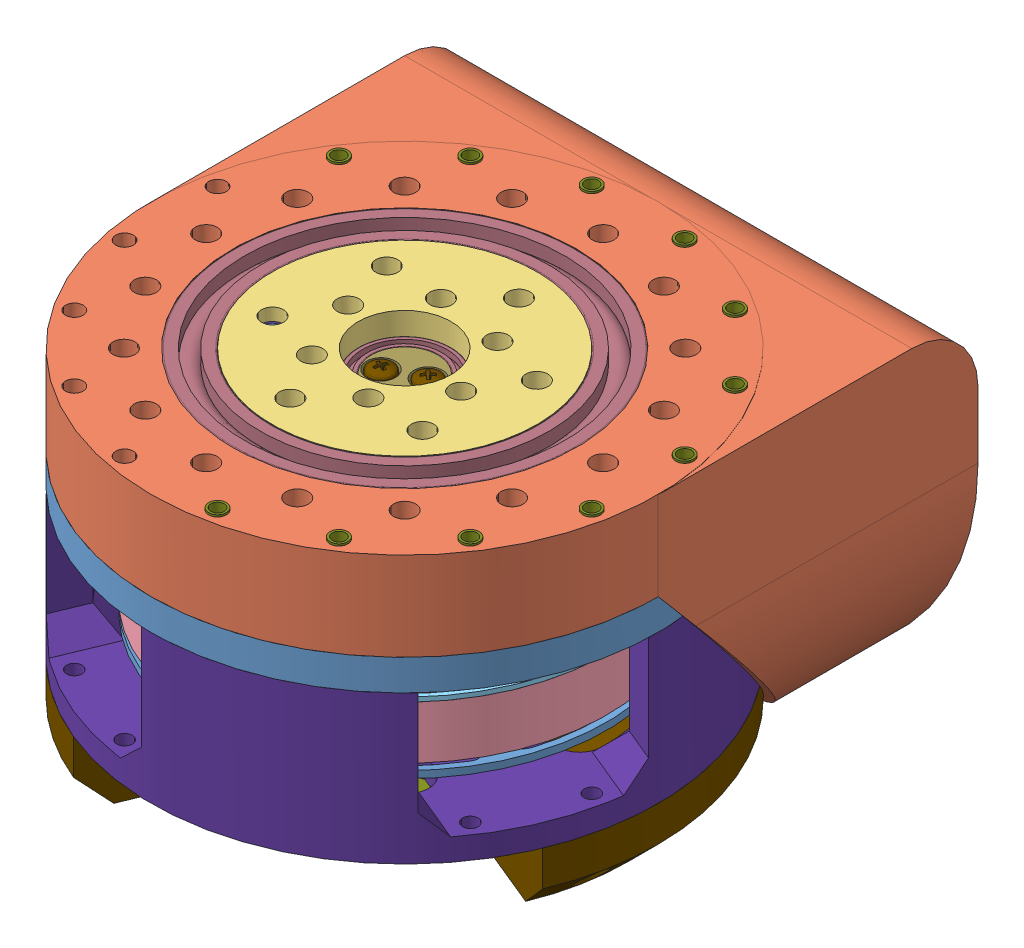
SolidWorks assembly Cycloidal_v3, configuration Default. Lengths in mm. (continued)
Components (placement in the parent): (continued)
- foc-motor-controller.step-1: foc-motor-controller.step [Default] at (47.267 33.7573 89.1587) x (-0.382683 0 -0.92388) z (0 -1 0) size (57.23 50 8.13) (continued)
  - R_0603_1608Metric.step-20: R_0603_1608Metric.step [Default] at (16 -17.8 1.595) x (0 1 0) z (0 0 1) size (1.6 0.8 0.45)
  - Texas_S-PVSON-N8.step-1: Texas_S-PVSON-N8.step [Default] at (-14.4105 -13.7 1.595) x (-1 0 0) z (0 0 1) size (3 2.98 0.92)
  - C_1206_3216Metric.step-14: C_1206_3216Metric.step [Default] at (21 -2.9 1.595) x (0.707107 -0.707107 0) z (0 0 1) size (3.2 1.6 1.6)
  - C_0603_1608Metric.step-24: C_0603_1608Metric.step [Default] at (-5.9 -16.6 1.595) x (0 1 0) z (0 0 1) size (1.6 0.8 0.8)
  - C_0603_1608Metric.step-25: C_0603_1608Metric.step [Default] at (-3.1 -14.1 1.595) size (1.6 0.8 0.8)
  - R_0603_1608Metric.step-21: R_0603_1608Metric.step [Default] at (7.2 -7.375 1.595) x (0 -1 0) z (0 0 1) size (1.6 0.8 0.45)
  - C_1206_3216Metric.step-15: C_1206_3216Metric.step [Default] at (-0.7 11 1.595) x (0 1 0) z (0 0 1) size (3.2 1.6 1.6)
  - LQFP-64_10x10mm_P0.5mm.step-1: LQFP-64_10x10mm_P0.5mm.step [Default] at (-7 -4.5 1.595) x (-1 0 0) z (0 0 1) size (12 12 1.5)
  - C_0805_2012Metric.step-2: C_0805_2012Metric.step [Default] at (23.35 -17 1.595) x (-1 0 0) z (0 0 1) size (2 1.25 1.25)
  - C_0603_1608Metric.step-26: C_0603_1608Metric.step [Default] at (10.8 -16.8 1.595) x (0 -1 0) z (0 0 1) size (1.6 0.8 0.8)
  - R_0603_1608Metric.step-22: R_0603_1608Metric.step [Default] at (17.5 -17.8 1.595) x (0 -1 0) z (0 0 1) size (1.6 0.8 0.45)
  - C_1206_3216Metric.step-16: C_1206_3216Metric.step [Default] at (20.3 11 1.595) x (0 1 0) z (0 0 1) size (3.2 1.6 1.6)
  - R_0603_1608Metric.step-23: R_0603_1608Metric.step [Default] at (9.2 -16.8 1.595) x (0 -1 0) z (0 0 1) size (1.6 0.8 0.45)
  - C_1206_3216Metric.step-17: C_1206_3216Metric.step [Default] at (-10 11 1.595) x (0 1 0) z (0 0 1) size (3.2 1.6 1.6)
  - R_0603_1608Metric.step-24: R_0603_1608Metric.step [Default] at (17.8 -15.2 1.595) size (1.6 0.8 0.45)
  - C_1206_3216Metric.step-18: C_1206_3216Metric.step [Default] at (19.9 2.6 1.595) x (-0.707107 0.707107 0) z (0 0 1) size (3.2 1.6 1.6)
  - C_0603_1608Metric.step-27: C_0603_1608Metric.step [Default] at (13.4 -7.375 1.595) x (0 -1 0) z (0 0 1) size (1.6 0.8 0.8)
  - R_0603_1608Metric.step-25: R_0603_1608Metric.step [Default] at (8.7 -7.375 1.595) x (0 -1 0) z (0 0 1) size (1.6 0.8 0.45)
  - PQFN-8-EP_6x5mm_P1.27mm_Generic.step-1: PQFN-8-EP_6x5mm_P1.27mm_Generic.step [Default] at (4.9 14.4 -0.085) x (0 1 0) z (0 0 -1) size (6.15 5.15 1.09)
  - C_0805_2012Metric.step-3: C_0805_2012Metric.step [Default] at (-3 8.9 -0.085) x (0 1 0) z (0 0 -1) size (2 1.25 1.25)
  - C_0603_1608Metric.step-28: C_0603_1608Metric.step [Default] at (1.5 -4.3 -0.085) x (0 1 0) z (0 0 -1) size (1.6 0.8 0.8)
  - R_2512_6332Metric.step-1: R_2512_6332Metric.step [Default] at (2.1 8.6 -0.085) x (-1 0 0) z (0 0 -1) size (6.3 3.2 0.6)
  - C_0805_2012Metric.step-4: C_0805_2012Metric.step [Default] at (18.8 8.9 -0.085) x (0 1 0) z (0 0 -1) size (2 1.25 1.25)
  - C_0805_2012Metric.step-5: C_0805_2012Metric.step [Default] at (-5.2 8.901 -0.085) x (0 1 0) z (0 0 -1) size (2 1.25 1.25)
  - PQFN-8-EP_6x5mm_P1.27mm_Generic.step-2: PQFN-8-EP_6x5mm_P1.27mm_Generic.step [Default] at (16.9 14.6 -0.085) x (0 -1 0) z (0 0 -1) size (6.15 5.15 1.09)
  - PQFN-8-EP_6x5mm_P1.27mm_Generic.step-3: PQFN-8-EP_6x5mm_P1.27mm_Generic.step [Default] at (-1.1 14.6 -0.085) x (0 -1 0) z (0 0 -1) size (6.15 5.15 1.09)
  - R_0603_1608Metric.step-26: R_0603_1608Metric.step [Default] at (8.2 8.8 -0.085) x (0 1 0) z (0 0 -1) size (1.6 0.8 0.45)
  - R_2512_6332Metric.step-2: R_2512_6332Metric.step [Default] at (-10.3 8.601 -0.085) x (1 0 0) z (0 0 -1) size (6.3 3.2 0.6)
  - TSSOP-16_4.4x5mm_P0.65mm.step-1: TSSOP-16_4.4x5mm_P0.65mm.step [Default] at (0 0 -0.085) x (-1 0 0) z (0 0 -1) size (6.4 5 1.1)
  - C_0603_1608Metric.step-29: C_0603_1608Metric.step [Default] at (0 -4.25 -0.085) x (0 1 0) z (0 0 -1) size (1.6 0.8 0.8)
  - PQFN-8-EP_6x5mm_P1.27mm_Generic.step-4: PQFN-8-EP_6x5mm_P1.27mm_Generic.step [Default] at (10.9 14.4 -0.085) x (0 1 0) z (0 0 -1) size (6.15 5.15 1.09)
  - R_2512_6332Metric.step-3: R_2512_6332Metric.step [Default] at (13.7 8.6 -0.085) x (1 0 0) z (0 0 -1) size (6.3 3.2 0.6)
  - PQFN-8-EP_6x5mm_P1.27mm_Generic.step-5: PQFN-8-EP_6x5mm_P1.27mm_Generic.step [Default] at (-13.1 14.401 -0.085) x (0 1 0) z (0 0 -1) size (6.15 5.15 1.09)
  - C_0603_1608Metric.step-30: C_0603_1608Metric.step [Default] at (-1.5 -4.3 -0.085) x (0 -1 0) z (0 0 -1) size (1.6 0.8 0.8)
  - PQFN-8-EP_6x5mm_P1.27mm_Generic.step-6: PQFN-8-EP_6x5mm_P1.27mm_Generic.step [Default] at (-7.1 14.601 -0.085) x (0 -1 0) z (0 0 -1) size (6.15 5.15 1.09)
  - foc-motor-controller_PCB.step-1: foc-motor-controller_PCB.step [Default] at origin size (50 50 1.51)
- hex nut style 1 gradeab_iso-1: hex nut style 1 gradeab_iso [ISO - 4032 - M3 - W - N] at (35.6313 33.7573 117.2498) x (1 0 0) z (0 -1 0) size (5.5 6.35 2.4)
- Cycloidal_Discs_8308-1: Cycloidal_Discs_8308 [Default] at (15.2211 42.227 25.7022) x (0.993378 0 0.114894) z (-0.114894 0 0.993378) size (79.25 5 79.73)
  - Cycloidal_Discs-1: Cycloidal_Discs [Default] at (38.3081 39.5303 58.0959) size (79.25 5 79.73)
  - radial ball bearing_68_iso-1: radial ball bearing_68_iso [ISO 15 RBB - 274 - 14,SI,NC,14_68] at (18.3896 43.2803 46.5959) x (0 1 0) z (0 0 1) size (2.5 7 7)
  - radial ball bearing_68_iso-2: radial ball bearing_68_iso [ISO 15 RBB - 274 - 14,SI,NC,14_68] at (38.3081 43.2803 81.0959) x (0 1 0) z (0 0 1) size (2.5 7 7)
  - radial ball bearing_68_iso-3: radial ball bearing_68_iso [ISO 15 RBB - 274 - 14,SI,NC,14_68] at (18.3896 43.2803 69.5959) x (0 1 0) z (0 0 1) size (2.5 7 7)
  - radial ball bearing_68_iso-4: radial ball bearing_68_iso [ISO 15 RBB - 274 - 14,SI,NC,14_68] at (38.3081 43.2803 35.0959) x (0 1 0) z (0 0 1) size (2.5 7 7)
  - radial ball bearing_68_iso-5: radial ball bearing_68_iso [ISO 15 RBB - 274 - 14,SI,NC,14_68] at (58.2267 43.2803 69.5959) x (0 1 0) z (0 0 1) size (2.5 7 7)
  - radial ball bearing_68_iso-6: radial ball bearing_68_iso [ISO 15 RBB - 274 - 14,SI,NC,14_68] at (58.2267 43.2803 46.5959) x (0 1 0) z (0 0 1) size (2.5 7 7)
- Cycloidal_Discs_8308-2: Cycloidal_Discs_8308 [Default] at (93.221 37.227 37.6663) x (0.275609 0 0.96127) z (-0.96127 0 0.275609) size (79.25 5 79.73)
  - Cycloidal_Discs-1: Cycloidal_Discs [Default] at (38.3081 39.5303 58.0959) size (79.25 5 79.73)
  - radial ball bearing_68_iso-1: radial ball bearing_68_iso [ISO 15 RBB - 274 - 14,SI,NC,14_68] at (18.3896 43.2803 46.5959) x (0 1 0) z (0 0 1) size (2.5 7 7)
  - radial ball bearing_68_iso-2: radial ball bearing_68_iso [ISO 15 RBB - 274 - 14,SI,NC,14_68] at (38.3081 43.2803 81.0959) x (0 1 0) z (0 0 1) size (2.5 7 7)
  - radial ball bearing_68_iso-3: radial ball bearing_68_iso [ISO 15 RBB - 274 - 14,SI,NC,14_68] at (18.3896 43.2803 69.5959) x (0 1 0) z (0 0 1) size (2.5 7 7)
  - radial ball bearing_68_iso-4: radial ball bearing_68_iso [ISO 15 RBB - 274 - 14,SI,NC,14_68] at (38.3081 43.2803 35.0959) x (0 1 0) z (0 0 1) size (2.5 7 7)
  - radial ball bearing_68_iso-5: radial ball bearing_68_iso [ISO 15 RBB - 274 - 14,SI,NC,14_68] at (58.2267 43.2803 69.5959) x (0 1 0) z (0 0 1) size (2.5 7 7)
  - radial ball bearing_68_iso-6: radial ball bearing_68_iso [ISO 15 RBB - 274 - 14,SI,NC,14_68] at (58.2267 43.2803 46.5959) x (0 1 0) z (0 0 1) size (2.5 7 7)
- m6-1: m6 [Default] at (25.9649 93.9895 97.8316) x (-0.80367 0 -0.595076) z (-0.595076 0 0.80367) size (6 16 6)
- Motor_Cover_v2-2: Motor_Cover_v2 [Default] at (47.267 36.1573 89.1587) x (-0.92388 0 -0.382683) z (0.382683 0 -0.92388) size (115 33.6 115)
- driver_cover-1: driver_cover [Default] at (47.267 36.1573 89.1587) x (-0.384295 0 -0.92321) z (-0.92321 0 0.384295) size (81.32 15 115)
- Base_plate_2-1: Base_plate_2 [Default] at (47.267 69.7573 89.1587) size (115 7 115)
- Cover_new-1: Cover_new [Default] at (47.267 86.8173 89.1587) size (115 87.56 130)
- Output_Shaft_D30-1: Output_Shaft_D30 [Default] at (47.267 86.8173 89.1587) x (0.990637 0 0.136524) z (-0.136524 0 0.990637) size (60 10 60)
Mates (geometry in assembly coordinates):
- Coincident1: coincident anti-aligned: plane of motor-X83008S.stp-1/outrunner.stp-1 through (31.9426 69.7573 58.2489) normal (0 1 0); plane of Base_Plate-1 through (47.267 69.7573 89.1587) normal (0 -1 0)
- Concentric1: concentric anti-aligned: line of motor-X83008S.stp-1/outrunner.stp-1 through (40.3821 64.2573 75.2717) axis (0 1 0); cylinder of Base_Plate-1 through (40.3821 76.7573 75.2717) axis (0 -1 0) radius 1.5
- Concentric2: concentric anti-aligned: cylinder of motor-X83008S.stp-1/shaft.stp-1 through (47.267 69.7573 89.1587) axis (0 1 0) radius 1.5; line of Base_Plate-1 through (47.267 76.7573 89.1587) axis (0 -1 0)
- Coincident2: coincident anti-aligned: plane of Base_Plate-1 through (47.267 76.7573 89.1587) normal (0 1 0); plane of Eccentric_Shaft-1/Eccentric_Shaft_bot-1 through (47.9333 76.7573 90.5026) normal (0 -1 0)
- Concentric78: concentric anti-aligned: cylinder of Base_Plate-1 through (47.267 76.7573 89.1587) axis (0 -1 0) radius 20; cylinder of radial ball bearing_68_iso-40 through (47.267 52.6198 89.1587) axis (0 1 0) radius 20
- Concentric14151: concentric aligned: cylinder of m13_bearing-2/m6-1 through (64.4877 86.8573 130.7332) axis (0 1 0) radius 2; cylinder of M4x6x5.5_brass_insert-20 through (64.4877 86.8573 130.7332) axis (0 1 0) radius 2
- Concentric14161: concentric aligned: cylinder of m13_bearing-11/m6-1 through (47.267 86.8573 134.1587) axis (0 1 0) radius 2; cylinder of M4x6x5.5_brass_insert-21 through (47.267 86.8573 134.1587) axis (0 1 0) radius 2
- Concentric14171: concentric aligned: cylinder of m13_bearing-1/m6-1 through (15.4472 86.8573 57.3389) axis (0 1 0) radius 2; cylinder of M4x6x5.5_brass_insert-22 through (15.4472 86.8573 57.3389) axis (0 1 0) radius 2
- Concentric14181: concentric aligned: cylinder of m13_bearing-6/m6-1 through (30.0462 86.8573 47.5841) axis (0 1 0) radius 2; cylinder of M4x6x5.5_brass_insert-23 through (30.0462 86.8573 47.5841) axis (0 1 0) radius 2
- Concentric14191: concentric aligned: cylinder of m13_bearing-12/m6-1 through (79.0868 86.8573 120.9785) axis (0 1 0) radius 2; cylinder of M4x6x5.5_brass_insert-24 through (79.0868 98.8014 120.9785) axis (0 1 0) radius 2.3
- Concentric14201: concentric aligned: cylinder of m13_bearing-5/m6-1 through (88.8416 86.8573 106.3794) axis (0 1 0) radius 2; cylinder of M4x6x5.5_brass_insert-25 through (88.8416 86.8573 106.3794) axis (0 1 0) radius 2
- Concentric14211: concentric aligned: cylinder of m13_bearing-4/m6-1 through (92.267 86.7573 89.1587) axis (0 1 0) radius 2; cylinder of M4x6x5.5_brass_insert-26 through (92.267 86.8573 89.1587) axis (0 1 0) radius 2
- Concentric14221: concentric aligned: cylinder of m13_bearing-9/m6-1 through (88.8416 86.8573 71.9379) axis (0 1 0) radius 2; cylinder of M4x6x5.5_brass_insert-27 through (88.8416 86.8573 71.9379) axis (0 1 0) radius 2
- Concentric14241: concentric aligned: cylinder of m13_bearing-7/m6-1 through (64.4877 86.8573 47.5841) axis (0 1 0) radius 2; cylinder of M4x6x5.5_brass_insert-29 through (64.4877 86.8573 47.5841) axis (0 1 0) radius 2
- Concentric14251: concentric aligned: cylinder of m13_bearing-3/m6-1 through (47.267 86.8573 44.1587) axis (0 1 0) radius 2; cylinder of M4x6x5.5_brass_insert-31 through (47.267 86.8573 44.1587) axis (0 1 0) radius 2
- Coincident1447: coincident anti-aligned: plane of m13_bearing-2/m6-1 through (64.4877 86.8573 130.7332) normal (0 1 0); plane of M4x6x5.5_brass_insert-20 through (64.4877 86.8573 130.7332) normal (0 -1 0)
- Coincident1458: coincident aligned: plane of M4x6x5.5_brass_insert-20 through (62.6232 92.8573 132.3986) normal (0 1 0); plane of M4x6x5.5_brass_insert-21 through (45.4024 92.8573 135.824) normal (0 1 0)
- Coincident1459: coincident aligned: plane of M4x6x5.5_brass_insert-20 through (62.6232 92.8573 132.3986) normal (0 1 0); plane of M4x6x5.5_brass_insert-22 through (17.0054 92.8573 59.2938) normal (0 1 0)
- Coincident1460: coincident aligned: plane of M4x6x5.5_brass_insert-20 through (62.6232 92.8573 132.3986) normal (0 1 0); plane of M4x6x5.5_brass_insert-23 through (31.6045 92.8573 49.5391) normal (0 1 0)
- Coincident1461: coincident aligned: plane of M4x6x5.5_brass_insert-20 through (62.6232 92.8573 132.3986) normal (0 1 0); plane of M4x6x5.5_brass_insert-31 through (46.7161 92.8573 46.5972) normal (0 1 0)
- Coincident1462: coincident aligned: plane of M4x6x5.5_brass_insert-20 through (62.6232 92.8573 132.3986) normal (0 1 0); plane of M4x6x5.5_brass_insert-29 through (64.1304 92.8573 50.0584) normal (0 1 0)
- Coincident1463: coincident aligned: plane of M4x6x5.5_brass_insert-20 through (62.6232 92.8573 132.3986) normal (0 1 0); plane of M4x6x5.5_brass_insert-28 through (79.0868 92.8573 57.3389) normal (0 1 0)
- Coincident1464: coincident aligned: plane of M4x6x5.5_brass_insert-20 through (62.6232 92.8573 132.3986) normal (0 1 0); plane of M4x6x5.5_brass_insert-27 through (86.977 92.8573 73.6032) normal (0 1 0)
- Coincident1465: coincident aligned: plane of M4x6x5.5_brass_insert-20 through (62.6232 92.8573 132.3986) normal (0 1 0); plane of M4x6x5.5_brass_insert-26 through (90.4024 92.8573 90.824) normal (0 1 0)
- Coincident1466: coincident aligned: plane of M4x6x5.5_brass_insert-20 through (62.6232 92.8573 132.3986) normal (0 1 0); plane of M4x6x5.5_brass_insert-25 through (86.977 92.8573 108.0448) normal (0 1 0)
- Coincident1467: coincident aligned: plane of M4x6x5.5_brass_insert-20 through (62.6232 92.8573 132.3986) normal (0 1 0); plane of M4x6x5.5_brass_insert-24 through (80.4417 92.8573 123.0795) normal (0 1 0)
- Concentric1426: concentric aligned: cylinder of pan cross head_am-1 through (50.8507 118.0573 87.3819) axis (0 1 0) radius 1.5; line of Eccentric_Shaft-1/Eccentric_Shaft_top-1 through (50.8507 90.2573 87.3819) axis (0 1 0)
- Coincident1468: coincident anti-aligned: plane of Eccentric_Shaft-1/Eccentric_Shaft_top-1 through (43.6832 90.2573 90.9354) normal (0 1 0); plane of pan cross head_am-1 through (51.8449 90.2573 86.2587) normal (0 -1 0)
- Concentric14281: concentric aligned: cylinder of pan cross head_am-3 through (43.6832 118.0573 90.9354) axis (0 1 0) radius 2.8; cylinder of Eccentric_Shaft-1/Eccentric_Shaft_top-1 through (43.6832 86.7573 90.9354) axis (0 1 0) radius 1.5
- Coincident14701: coincident anti-aligned: plane of Eccentric_Shaft-1/Eccentric_Shaft_top-1 through (50.8507 90.2573 87.3819) normal (0 1 0); plane of pan cross head_am-3 through (44.1937 90.2573 89.5249) normal (0 -1 0)
- Concentric1437: concentric anti-aligned: cylinder of Base_Plate-1 through (50.8507 76.7573 87.3819) axis (0 -1 0) radius 2; cylinder of M3x4x4.2_brass_insert-22 through (50.8507 74.6594 87.3819) axis (0 1 0) radius 1.5
- Coincident1479: coincident aligned: plane of Base_Plate-1 through (47.267 69.7573 89.1587) normal (0 -1 0); plane of M3x4x4.2_brass_insert-22 through (52.3275 69.7573 87.1187) normal (0 -1 0)
- Concentric1438: concentric anti-aligned: cylinder of Base_Plate-1 through (43.6832 76.7573 90.9354) axis (0 -1 0) radius 2; cylinder of M3x4x4.2_brass_insert-23 through (43.6832 74.6594 90.9354) axis (0 1 0) radius 1.5
- Coincident1480: coincident aligned: plane of Base_Plate-1 through (47.267 69.7573 89.1587) normal (0 -1 0); plane of M3x4x4.2_brass_insert-23 through (45.1602 69.7573 90.6733) normal (0 -1 0)
- Concentric1439: concentric anti-aligned: cylinder of Base_Plate-1 through (33.38 76.7573 96.0435) axis (0 -1 0) radius 1.5; cylinder of pan cross head_am-4 through (33.38 103.0573 96.0435) axis (0 1 0) radius 1.5
- Coincident1481: coincident anti-aligned: plane of Base_Plate-1 through (33.38 75.2573 96.0435) normal (0 1 0); plane of pan cross head_am-4 through (34.88 75.2573 96.0435) normal (0 -1 0)
- Concentric14401: concentric anti-aligned: cylinder of Base_Plate-1 through (61.154 76.7573 82.2738) axis (0 -1 0) radius 1.5; cylinder of pan cross head_am-5 through (61.154 103.0573 82.2738) axis (0 1 0) radius 2.8
- Coincident14821: coincident anti-aligned: plane of Base_Plate-1 through (61.154 75.2573 82.2738) normal (0 1 0); plane of pan cross head_am-5 through (62.654 75.2573 82.2738) normal (0 -1 0)
- Concentric1445021: concentric anti-aligned: cylinder of Base_Plate-1 through (54.1518 76.7573 103.0457) axis (0 -1 0) radius 1.5; cylinder of pan cross head_am-6 through (54.1518 103.0573 103.0457) axis (0 1 0) radius 2.8
- Coincident1486621: coincident anti-aligned: plane of Base_Plate-1 through (54.1518 75.2573 103.0457) normal (0 1 0); plane of pan cross head_am-6 through (55.6518 75.2573 103.0457) normal (0 -1 0)
- Concentric1445031: concentric anti-aligned: cylinder of Base_Plate-1 through (40.3821 76.7573 75.2717) axis (0 -1 0) radius 1.5; cylinder of pan cross head_am-7 through (40.3821 103.0573 75.2717) axis (0 1 0) radius 2.8
- Coincident1486631: coincident anti-aligned: plane of Base_Plate-1 through (40.3821 75.2573 75.2717) normal (0 1 0); plane of pan cross head_am-7 through (41.8821 75.2573 75.2717) normal (0 -1 0)
- Concentric1445035: concentric anti-aligned: cylinder of Eccentric_Shaft-1/Eccentric_Shaft_bot-1 through (47.9333 81.7573 90.5026) axis (0 -1 0) radius 7.5; cylinder of radial ball bearing_68_iso-46 through (47.9333 59.1198 90.5026) axis (0 1 0) radius 7.5
- Coincident1486648: coincident aligned: plane of Eccentric_Shaft-1/Eccentric_Shaft_bot-1 through (47.9333 81.7573 90.5026) normal (0 1 0); plane of radial ball bearing_68_iso-46 through (40.2333 81.7573 90.5075) normal (0 1 0)
- Concentric1445036: concentric anti-aligned: cylinder of Eccentric_Shaft-1/Eccentric_Shaft_bot-2 through (46.6007 86.7573 87.8148) axis (0 -1 0) radius 7.5; cylinder of radial ball bearing_68_iso-44 through (46.6007 64.1198 87.8148) axis (0 1 0) radius 7.5
- Coincident1486649: coincident aligned: plane of Eccentric_Shaft-1/Eccentric_Shaft_bot-2 through (46.6007 82.7573 87.8148) normal (0 1 0); circle of radial ball bearing_68_iso-44
- Concentric1445037: concentric anti-aligned: cylinder of Eccentric_Shaft-1/Eccentric_Shaft_top-1 through (47.267 91.7573 89.1587) axis (0 -1 0) radius 7.5; cylinder of radial ball bearing_68_iso-45 through (47.267 69.1198 89.1587) axis (0 1 0) radius 7.5
- Concentric1445038: concentric anti-aligned: cylinder of Base_Plate-1 through (47.267 76.7573 89.1587) axis (0 -1 0) radius 20; cylinder of radial ball bearing_68_iso-40 through (47.267 52.6198 89.1587) axis (0 1 0) radius 20
- Coincident1486655: coincident anti-aligned: plane of Eccentric_Shaft-1/Eccentric_Shaft_top-1 through (47.267 87.7573 89.1587) normal (0 1 0); plane of radial ball bearing_68_iso-45 through (47.5372 87.7573 97.5543) normal (0 -1 0)
- Concentric1445042: concentric anti-aligned: cylinder of Base_Plate-1 through (43.6832 76.7573 90.9354) axis (0 -1 0) radius 2; cylinder of Eccentric_Shaft-1/Eccentric_Shaft_bot-1 through (43.6832 76.7573 90.9354) axis (0 1 0) radius 1.5
- Concentric1445043: concentric aligned: cylinder of Eccentric_Shaft-1/Eccentric_Shaft_bot-1 through (50.8507 76.7573 87.3819) axis (0 1 0) radius 1.5; cylinder of M3x4x4.2_brass_insert-22 through (50.8507 74.6594 87.3819) axis (0 1 0) radius 1.5
- Concentric1445052: concentric aligned: circle of m13_bearing-31/m6-1; cylinder of M4x6x5.5_brass_insert-47 through (5.6924 92.8573 71.9379) axis (0 -1 0) radius 2
- Concentric1445056: concentric aligned: circle of m13_bearing-32/m6-1; cylinder of M4x6x5.5_brass_insert-48 through (2.267 92.8573 89.1587) axis (0 -1 0) radius 2
- Coincident1486681: coincident anti-aligned: plane of m13_bearing-1/m6-1 through (15.4472 92.8573 57.3389) normal (0 1 0); circle of M4x6x5.5_brass_insert-47
- Concentric1445063: concentric aligned: cylinder of m13_bearing-34/m6-1 through (30.0462 87.0073 130.7332) axis (0 1 0) radius 2; cylinder of M4x6x5.5_brass_insert-51 through (30.0462 87.0073 130.7332) axis (0 1 0) radius 2
- Coincident1486686: coincident aligned: plane of m13_bearing-36/m6-1 through (5.6924 93.0073 106.3794) normal (0 1 0); circle of M4x6x5.5_brass_insert-49
- Coincident1486687: coincident anti-aligned: plane of m13_bearing-32/m6-1 through (2.267 92.8573 89.1587) normal (0 1 0); circle of M4x6x5.5_brass_insert-48
- Coincident1486688: coincident aligned: plane of m13_bearing-35/m6-1 through (15.4472 92.8573 120.9785) normal (0 1 0); circle of M4x6x5.5_brass_insert-50
- Coincident1486690: coincident aligned: plane of m13_bearing-34/m6-1 through (30.0462 93.0073 130.7332) normal (0 1 0); circle of M4x6x5.5_brass_insert-51
- Coincident1486692: coincident anti-aligned: plane of foc-motor-controller.step-1/foc-motor-controller_PCB.step-1 through (47.267 33.7573 89.1587) normal (0 1 0); plane of hex nut style 1 gradeab_iso-1 through (35.6313 33.7573 120.4252) normal (0 -1 0)
- Concentric14450545: concentric anti-aligned: cylinder of radial ball bearing_68_iso-46 through (47.9333 59.1198 90.5026) axis (0 1 0) radius 10.5; cylinder of Cycloidal_Discs_8308-2/Cycloidal_Discs-1 through (47.9333 81.7573 90.5026) axis (0 -1 0) radius 10.5
- Coincident1486693: coincident aligned: plane of radial ball bearing_68_iso-46 through (37.6333 81.7573 90.5092) normal (0 1 0); plane of Cycloidal_Discs_8308-2/Cycloidal_Discs-1 through (84.855 81.7573 80.0906) normal (0 1 0)
- Concentric14450546: concentric anti-aligned: cylinder of radial ball bearing_68_iso-44 through (46.6007 64.1198 87.8148) axis (0 1 0) radius 10.5; cylinder of Cycloidal_Discs_8308-1/Cycloidal_Discs-1 through (46.6007 86.7573 87.8148) axis (0 -1 0) radius 10.5
- Coincident1486694: coincident aligned: plane of radial ball bearing_68_iso-44 through (53.8022 86.7573 80.4508) normal (0 1 0); plane of Cycloidal_Discs_8308-1/Cycloidal_Discs-1 through (51.1744 86.7573 49.7266) normal (0 1 0)
- Concentric14450547: concentric anti-aligned: cylinder of M4x6x5.5_brass_insert-6 through (25.9649 93.9895 97.8316) axis (0 -1 0) radius 2; cylinder of m6-1 through (25.9649 87.9895 97.8316) axis (0 1 0) radius 2
- Coincident1486695: coincident anti-aligned: circle of M4x6x5.5_brass_insert-6; plane of m6-1 through (25.9649 87.9895 97.8316) normal (0 1 0)
- Tangent1: tangent aligned: cylinder of Cycloidal_Discs_8308-1/radial ball bearing_68_iso-3 through (25.4928 64.8698 96.9501) axis (0 1 0) radius 2; cylinder of m6-1 through (25.9649 77.9895 97.8316) axis (0 1 0) radius 3
- Tangent3: tangent aligned: cylinder of Cycloidal_Discs_8308-2/radial ball bearing_68_iso-2 through (25.8241 59.8698 96.8416) axis (0 1 0) radius 2; cylinder of m6-1 through (25.9649 77.9895 97.8316) axis (0 1 0) radius 3
- Concentric14450559: concentric anti-aligned: cylinder of foc-motor-controller.step-1/foc-motor-controller_PCB.step-1 through (58.9027 33.8033 61.0676) axis (0 1 0) radius 1.6; cylinder of Motor_Cover_v2-2 through (58.9027 86.1573 61.0676) axis (0 -1 0) radius 1.5
- Concentric14450560: concentric anti-aligned: circle of foc-motor-controller.step-1/foc-motor-controller_PCB.step-1; cylinder of Motor_Cover_v2-2 through (35.6313 86.1573 117.2498) axis (0 -1 0) radius 1.5
- Coincident1486699: coincident anti-aligned: line of foc-motor-controller.step-1/foc-motor-controller_PCB.step-1 through (35.6313 32.2473 117.2498) axis (0 1 0); line of hex nut style 1 gradeab_iso-1 through (35.6313 35.9569 117.2498) axis (0 -1 0)
- Coincident1486700: coincident aligned: circle of hex nut style 1 gradeab_iso-1; plane of Motor_Cover_v2-2 through (47.267 36.1573 89.1587) normal (0 -1 0)
- Concentric14450561: concentric anti-aligned: cylinder of Motor_Cover_v2-2 through (47.267 69.7573 89.1587) axis (0 -1 0) radius 57.5; cylinder of driver_cover-1 through (47.267 21.1573 89.1587) axis (0 1 0) radius 57.5
- Coincident1486701: coincident anti-aligned: plane of Motor_Cover_v2-2 through (47.267 36.1573 89.1587) normal (0 -1 0); plane of driver_cover-1 through (47.267 36.1573 89.1587) normal (0 1 0)
- Concentric14450565: concentric aligned: cylinder of m13_bearing-36/m6-1 through (5.6924 87.0073 106.3794) axis (0 1 0) radius 2; cylinder of M4x6x5.5_brass_insert-49 through (5.6924 87.0073 106.3794) axis (0 1 0) radius 2
- Concentric14450566: concentric aligned: cylinder of Motor_Cover_v2-2 through (92.1663 86.1573 59.1579) axis (0 -1 0) radius 1.75; cylinder of driver_cover-1 through (92.1663 36.1573 59.1579) axis (0 -1 0) radius 1.75
- Concentric14450569: concentric anti-aligned: cylinder of Base_Plate-1 through (47.267 76.7573 89.1587) axis (0 -1 0) radius 20; cylinder of radial ball bearing_68_iso-40 through (47.267 52.6198 89.1587) axis (0 1 0) radius 20
- Concentric14450570: concentric aligned: cylinder of Motor_Cover_v2-2 through (47.267 69.7573 89.1587) axis (0 -1 0) radius 57.5; cylinder of Base_plate_2-1 through (47.267 76.7573 89.1587) axis (0 -1 0) radius 57.5
- Concentric14450571: concentric anti-aligned: cylinder of radial ball bearing_68_iso-40 through (47.267 52.6198 89.1587) axis (0 1 0) radius 26; cylinder of Base_plate_2-1 through (47.267 76.7573 89.1587) axis (0 -1 0) radius 57.5
- Coincident1486702: coincident anti-aligned: plane of Motor_Cover_v2-2 through (47.267 69.7573 89.1587) normal (0 1 0); plane of Base_plate_2-1 through (47.267 69.7573 89.1587) normal (0 -1 0)
- Concentric14450572: concentric anti-aligned: cylinder of m13_bearing-5/radial ball bearing_68_iso-1 through (88.8416 99.9948 106.3794) axis (0 -1 0) radius 6.5; circle of Base_plate_2-1
- Concentric14450573: concentric anti-aligned: cylinder of radial ball bearing_68_iso-39 through (47.267 71.1798 89.1587) axis (0 1 0) radius 39; cylinder of Base_plate_2-1 through (47.267 76.7573 89.1587) axis (0 -1 0) radius 57.5
- Coincident1486704: coincident anti-aligned: plane of Cycloidal_Discs_8308-2/Cycloidal_Discs-1 through (84.855 76.7573 80.0906) normal (0 -1 0); plane of Base_plate_2-1 through (47.267 76.7573 89.1587) normal (0 1 0)
- Concentric14450574: concentric aligned: cylinder of Base_plate_2-1 through (47.267 76.7573 89.1587) axis (0 -1 0) radius 57.5; cylinder of Cover_new-1 through (47.267 96.8173 89.1587) axis (0 -1 0) radius 57.5
- Concentric14450576: concentric anti-aligned: cylinder of m13_bearing-4/radial ball bearing_68_iso-2 through (92.267 104.8948 89.1587) axis (0 -1 0) radius 6.5; cylinder of Cover_new-1 through (92.267 76.7573 89.1587) axis (0 1 0) radius 7
- Concentric14450577: concentric anti-aligned: cylinder of m13_bearing-4/radial ball bearing_68_iso-2 through (92.267 104.8948 89.1587) axis (0 -1 0) radius 6.5; cylinder of Base_plate_2-1 through (92.267 75.7573 89.1587) axis (0 1 0) radius 5
- Coincident1486706: coincident anti-aligned: plane of m13_bearing-4/m6-1 through (92.267 76.7573 89.1587) normal (0 -1 0); plane of Base_plate_2-1 through (47.267 76.7573 89.1587) normal (0 1 0)
- Coincident1486707: coincident anti-aligned: plane of Base_plate_2-1 through (47.267 76.7573 89.1587) normal (0 1 0); plane of Cover_new-1 through (47.267 76.7573 89.1587) normal (0 -1 0)
- Concentric14450578: concentric aligned: cylinder of driver_cover-1 through (-5.6954 36.1573 99.6935) axis (0 -1 0) radius 1.75; cylinder of Base_plate_2-1 through (-5.6954 76.7573 99.6935) axis (0 -1 0) radius 1.75
- Coincident1486708: coincident aligned: plane of Cover_new-1 through (47.267 96.8173 89.1587) normal (0 1 0); plane of Output_Shaft_D30-1 through (47.267 96.8173 89.1587) normal (0 1 0)
- Concentric14450579: concentric anti-aligned: cylinder of radial ball bearing_68_iso-39 through (47.267 71.1798 89.1587) axis (0 1 0) radius 30; cylinder of Output_Shaft_D30-1 through (47.267 96.8173 89.1587) axis (0 -1 0) radius 30
- Concentric14450580: concentric aligned: cylinder of M4x6x5.5_brass_insert-6 through (25.9649 82.0455 97.8316) axis (0 -1 0) radius 2.5; cylinder of Output_Shaft_D30-1 through (25.9649 96.8173 97.8316) axis (0 -1 0) radius 2.5
